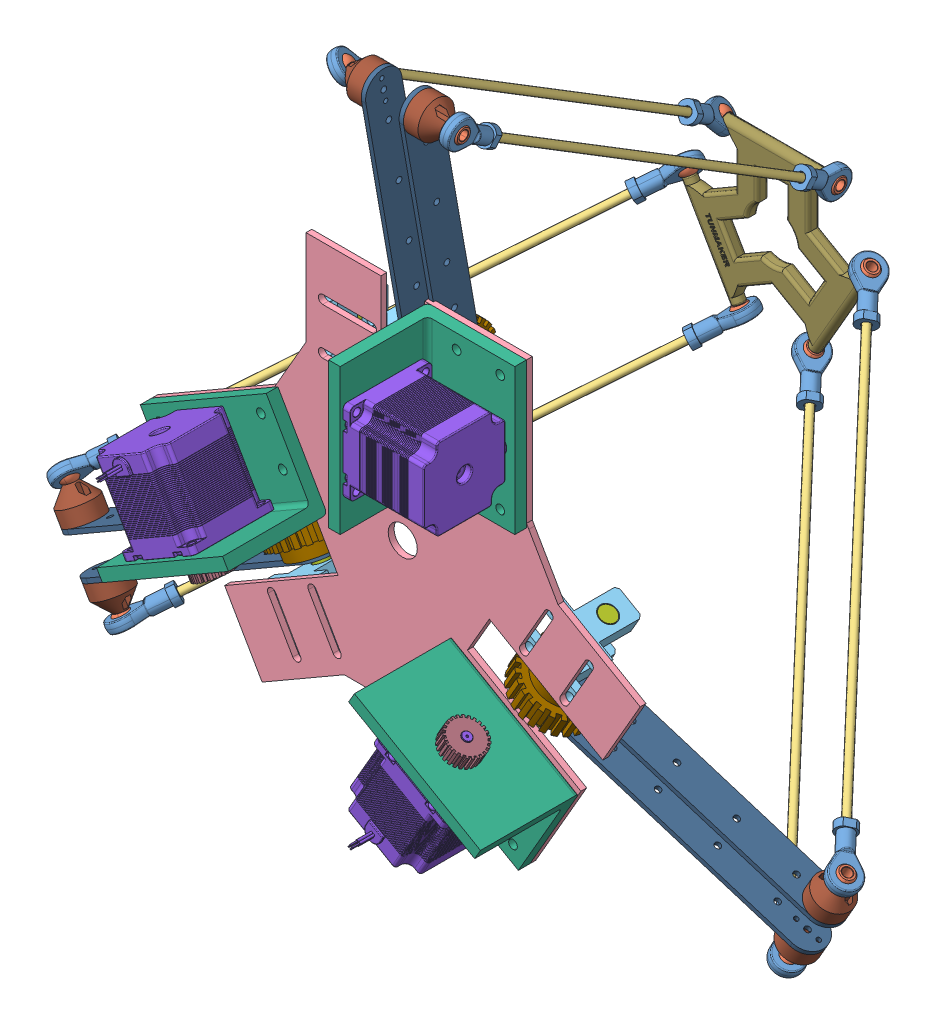
SolidWorks assembly deltabot+metal, configuration Default. Lengths in mm.
Overall size (531.43 463.37 392.64).
84 component instances, 13 part files, 0 mates.
Components (placement in the parent):
- deltabot+metal.stp-1: deltabot+metal.stp [Default] at origin size (531.43 463.37 392.64)
  - arm with joints v4.stp-1: arm with joints v4.stp [Default] at (0 -700 0) size (201.57 166.8 282.45)
    - RF_6-XE_MecMove.stp-1: RF_6-XE_MecMove.stp [Default] at (797.1961 -292.6027 -245.4013) size (39.77 32.89 44.28)
      - Component1.stp-1: Component1.stp [Default] at (-1006.4749 831.2054 216.1304) x (0.678851 0.338604 0.651543) z (0.528727 -0.841135 -0.113754) size (20 40 11)
      - Component2.stp-1: Component2.stp [Default] at (-1012.7729 825.9928 237.762) x (0.866025 0.5 0) z (-0.5 0.866025 0) size (12.7 12.7 9)
    - RF_6-XE_MecMove_1.stp-1: RF_6-XE_MecMove_1.stp [Default] at (137.5516 -501.3584 331.6266) size (39.77 32.89 44.28)
      - Component1.stp-1: Component1.stp [Default] at (-187.4437 1171.88 -595.5223) x (0.678851 0.338604 0.651543) z (-0.528727 0.841135 0.113754) size (20 40 11)
      - Component2.stp-1: Component2.stp [Default] at (-178.3751 1178.6922 -616.7328) x (0.836516 0.482963 0.258819) z (0.5 -0.866025 0) size (12.7 12.7 9)
    - connecting rod.stp-1: connecting rod.stp [Default] at (-415.8051 -153.3483 -567.1679) x (0.678851 0.338604 0.651543) z (0.509518 0.42171 -0.750034) size (5 5 300)
  - arm with joints v4_1.stp-1: arm with joints v4_1.stp [Default] at (0 -800 0) size (196.17 171.43 283.24)
    - RF_6-XE_MecMove_2.stp-1: RF_6-XE_MecMove_2.stp [Default] at (797.1961 -292.6027 -245.4013) size (34.38 37.52 45.07)
      - Component1.stp-1: Component1.stp [Default] at (-1045.4749 998.7554 216.1304) x (0.246638 0.763515 0.596837) z (0.824355 -0.489086 0.285015) size (20 40 11)
      - Component2.stp-1: Component2.stp [Default] at (-1051.7729 993.5428 237.762) x (0.866025 0.5 0) z (-0.5 0.866025 0) size (12.7 12.7 9)
    - RF_6-XE_MecMove_3.stp-1: RF_6-XE_MecMove_3.stp [Default] at (137.5516 -501.3584 331.6266) size (34.38 37.52 45.07)
      - Component1.stp-1: Component1.stp [Default] at (-226.4437 1339.43 -595.5223) x (0.246638 0.763515 0.596837) z (-0.824355 0.489086 -0.285015) size (20 40 11)
      - Component2.stp-1: Component2.stp [Default] at (-222.9163 1343.043 -592.8538) x (-0.836516 -0.482963 -0.258819) z (0.5 -0.866025 0) size (12.7 12.7 9)
    - connecting rod.stp-1: connecting rod.stp [Default] at (16.4032 -105.8427 -314.5592) x (0.246638 0.763515 0.596837) z (0.509518 0.42171 -0.750034) size (5 5 300)
  - arm with joints v4_2.stp-1: arm with joints v4_2.stp [Default] at (0 -900 0) size (236.66 169.54 252.51)
    - RF_6-XE_MecMove_4.stp-1: RF_6-XE_MecMove_4.stp [Default] at (797.1961 -292.6027 -245.4013) size (42.08 32.77 42.12)
      - Component1.stp-1: Component1.stp [Default] at (-554.93 1095.8279 187.6912) x (-0.588292 0.311209 0.746365) z (0.527669 0.847134 0.062688) size (20 40 11)
      - Component2.stp-1: Component2.stp [Default] at (-545.497 1089.4308 208.054) x (0.852869 -0.492404 -0.173648) z (0.5 0.866025 0) size (12.7 12.7 9)
    - RF_6-XE_MecMove_5.stp-1: RF_6-XE_MecMove_5.stp [Default] at (137.5516 -501.3584 331.6266) size (42.08 32.77 42.12)
      - Component1.stp-1: Component1.stp [Default] at (-86.969 1439.3187 -596.6034) x (-0.588292 0.311209 0.746365) z (-0.527669 -0.847134 -0.062688) size (20 40 11)
      - Component2.stp-1: Component2.stp [Default] at (-84.8414 1439.0413 -599.5694) x (-0.365998 0.211309 0.906308) z (-0.5 -0.866025 0) size (12.7 12.7 9)
    - connecting rod.stp-1: connecting rod.stp [Default] at (946.6115 1032.7546 -569.5657) x (-0.588292 0.311209 0.746365) z (-0.612762 0.430713 -0.662578) size (5 5 300)
  - arm with joints v4_3.stp-1: arm with joints v4_3.stp [Default] at (0 -1000 0) size (37.82 211.61 310.51)
    - RF_6-XE_MecMove_6.stp-1: RF_6-XE_MecMove_6.stp [Default] at (797.1961 -292.6027 -245.4013) size (15.43 39.54 44.57)
      - Component1.stp-1: Component1.stp [Default] at (-755.0673 1553.322 244.5695) x (0.084018 0.833371 -0.546291) z (0.993968 -0.108872 -0.013215) size (20 40 11)
      - Component2.stp-1: Component2.stp [Default] at (-754.1961 1557.8737 267.0944) x (0 -0.984808 -0.173648) z (1 0 0) size (12.7 12.7 9)
    - RF_6-XE_MecMove_7.stp-1: RF_6-XE_MecMove_7.stp [Default] at (137.5516 -501.3584 331.6266) size (15.43 39.54 44.57)
      - Component1.stp-1: Component1.stp [Default] at (-117.4731 1592.5657 -594.4413) x (0.084018 0.833371 -0.546291) z (-0.993968 0.108872 0.013215) size (20 40 11)
      - Component2.stp-1: Component2.stp [Default] at (-118.3444 1573.507 -604.7933) x (0 0 -1) z (1 0 0) size (12.7 12.7 9)
    - connecting rod.stp-1: connecting rod.stp [Default] at (511.5618 594.9454 382.7829) x (0.084018 0.833371 -0.546291) z (-0.070489 -0.541885 -0.837491) size (5 5 300)
  - arm with joints v4_4.stp-1: arm with joints v4_4.stp [Default] at (0 -1100 0) size (47.47 212.02 310.6)
    - RF_6-XE_MecMove_8.stp-1: RF_6-XE_MecMove_8.stp [Default] at (797.1961 -292.6027 -245.4013) size (25.08 39.95 44.66)
      - Component1.stp-1: Component1.stp [Default] at (-833.0673 1653.322 244.5695) x (0.753822 -0.578791 0.311051) z (-0.653287 -0.609394 0.449284) size (20 40 11)
      - Component2.stp-1: Component2.stp [Default] at (-832.1961 1662.1665 242.7486) x (0 -0.984808 -0.173648) z (-1 0 0) size (12.7 12.7 9)
    - RF_6-XE_MecMove_9.stp-1: RF_6-XE_MecMove_9.stp [Default] at (137.5516 -501.3584 331.6266) size (25.08 39.95 44.66)
      - Component1.stp-1: Component1.stp [Default] at (-195.4731 1692.5657 -594.4413) x (0.753822 -0.578791 0.311051) z (0.653287 0.609394 -0.449284) size (20 40 11)
      - Component2.stp-1: Component2.stp [Default] at (-196.3444 1673.507 -604.7933) x (0 0 -1) z (1 0 0) size (12.7 12.7 9)
    - connecting rod.stp-1: connecting rod.stp [Default] at (-931.6802 1451.4209 8.2253) x (0.753822 -0.578791 0.311051) z (-0.070489 -0.541885 -0.837491) size (5 5 300)
  - arm with joints v4_5.stp-1: arm with joints v4_5.stp [Default] at (0 -1200 0) size (236.83 168.87 252.83)
    - RF_6-XE_MecMove_10.stp-1: RF_6-XE_MecMove_10.stp [Default] at (797.1961 -292.6027 -245.4013) size (42.26 32.1 42.44)
      - Component1.stp-1: Component1.stp [Default] at (-593.93 1328.2779 187.6912) x (0.612958 -0.270161 -0.742493) z (-0.498804 -0.861103 -0.098465) size (20 40 11)
      - Component2.stp-1: Component2.stp [Default] at (-588.2147 1324.0272 183.7082) x (0.852869 -0.492404 -0.173648) z (-0.5 -0.866025 0) size (12.7 12.7 9)
    - RF_6-XE_MecMove_11.stp-1: RF_6-XE_MecMove_11.stp [Default] at (137.5516 -501.3584 331.6266) size (42.26 32.1 42.44)
      - Component1.stp-1: Component1.stp [Default] at (-125.969 1671.7687 -596.6034) x (0.612958 -0.270161 -0.742493) z (0.498804 0.861103 0.098465) size (20 40 11)
      - Component2.stp-1: Component2.stp [Default] at (-133.5432 1677.0926 -617.1539) x (-0.866025 0.5 0) z (0.5 0.866025 0) size (12.7 12.7 9)
    - connecting rod.stp-1: connecting rod.stp [Default] at (-511.4012 774.4489 423.7397) x (0.612958 -0.270161 -0.742493) z (-0.612762 0.430713 -0.662578) size (5 5 300)
  - Base.stp-1: Base.stp [Default] at origin size (335.56 298.61 4)
  - 12 mm rod alu support.stp-1: 12 mm rod alu support.stp [Default] at (98.916 13.3275 0) x (0.866025 -0.5 0) z (0 0 -1) size (42 12 35)
  - 12 mm rod alu support.stp-2: 12 mm rod alu support.stp [Default] at (-54.916 -62.8827 0) x (-0.866025 -0.5 0) z (0 0 -1) size (42 12 35)
  - 12 mm rod alu support.stp-3: 12 mm rod alu support.stp [Default] at (-80.2891 -102.9352 0) x (0.866025 0.5 0) z (0 0 -1) size (42 12 35)
  - 12 mm rod alu support.stp-4: 12 mm rod alu support.stp [Default] at (-20 121 0) x (0 -1 0) z (0 0 -1) size (42 12 35)
  - 12 mm rod alu support.stp-5: 12 mm rod alu support.stp [Default] at (-49 121 0) x (0 -1 0) z (0 0 -1) size (42 12 35)
  - 12 mm rod alu support.stp-6: 12 mm rod alu support.stp [Default] at (81.916 -16.1173 0) x (0.866025 -0.5 0) z (0 0 -1) size (42 12 35)
  - Stepper Mount.stp-1: Stepper Mount.stp [Default] at (258.4596 347.6652 0.886) x (0.866025 -0.5 0) z (0 0 1) size (100 68 68)
  - Stepper Mount.stp-2: Stepper Mount.stp [Default] at (171.8571 -397.6652 0.886) x (-0.866025 -0.5 0) z (0 0 1) size (100 68 68)
  - Stepper Mount.stp-3: Stepper Mount.stp [Default] at (-430.3167 50 0.886) x (0 1 0) z (0 0 1) size (100 68 68)
  - 12 mm axel.stp-1: 12 mm axel.stp [Default] at (-61 223.5554 -0.7002) x (0 -0.984808 -0.173648) z (0 -0.173648 0.984808) size (11 100 11)
  - 12 mm axel.stp-2: 12 mm axel.stp [Default] at (-39.8995 -21.9973 -0.7002) x (0.852869 -0.492404 -0.173648) z (0.150384 -0.086824 0.984808) size (11 100 11)
  - 12 mm axel.stp-3: 12 mm axel.stp [Default] at (-214.3814 -78.7398 -17.5515) x (0.866025 0.5 0) z (0 0 -1) size (11 100 11)
  - Stepper Motor length 56mm.stp-1: Stepper Motor length 56mm.stp [Default] at (-800.7521 882.2228 43.5) x (0.422618 0.906308 0) z (0 0 1) size (78.85 60.84 73.5)
  - Stepper Motor length 56mm.stp-2: Stepper Motor length 56mm.stp [Default] at (1164.4034 252.3603 43.5) x (0.573576 -0.819152 0) z (0 0 1) size (78.85 60.84 73.5)
  - Stepper Motor length 56mm.stp-3: Stepper Motor length 56mm.stp [Default] at (-363.6513 1334.5831 43.5) x (-0.996195 0.087156 0) z (0 0 -1) size (78.85 60.84 73.5)
  - pulley 50.stp-1: pulley 50.stp [Default] at (1 65.9551 177.8108) x (0 -0.173648 0.984808) z (-1 0 0) size (51 50.96 23)
  - pulley 50.stp-2: pulley 50.stp [Default] at (117.738 -67.3987 177.5254) x (0.150384 -0.086824 0.984808) z (0.5 0.866025 0) size (51 50.96 23)
  - pulley 50.stp-3: pulley 50.stp [Default] at (-87.0642 -50.8439 180.7174) x (0 0 1) z (0.5 -0.866025 0) size (51 50.96 23)
  - arm.stp-1: arm.stp [Default] at (242.9495 -126.4106 371.9297) x (-0.150384 0.086824 -0.984808) z (-0.5 -0.866025 0) size (25 195 3)
  - arm.stp-2: arm.stp [Default] at (103.2937 -79.2665 -447.6701) x (0.150384 -0.086824 0.984808) z (0.5 0.866025 0) size (25 195 3)
  - arm.stp-3: arm.stp [Default] at (-171.2256 -109.2494 -436.1217) x (0 0 1) z (0.5 -0.866025 0) size (25 195 3)
  - arm.stp-4: arm.stp [Default] at (18.5 273.6058 -411.9297) x (0 -0.173648 0.984808) z (-1 0 0) size (25 195 3)
  - arm.stp-5: arm.stp [Default] at (-184.2256 -86.7328 -436.1217) x (0 0 1) z (0.5 -0.866025 0) size (25 195 3)
  - arm.stp-6: arm.stp [Default] at (-7.5 273.6058 -411.9297) x (0 -0.173648 0.984808) z (-1 0 0) size (25 195 3)
  - Ball Top.stp-1: Ball Top.stp [Default] at (18.5 453.5434 278.0005) x (0 -0.984808 -0.173648) z (1 0 0) size (25 25 20)
  - Ball Top.stp-2: Ball Top.stp [Default] at (-10.5 534.1443 -179.1099) x (0 -0.984808 -0.173648) z (-1 0 0) size (25 25 20)
  - Ball Top.stp-3: Ball Top.stp [Default] at (-43.2107 -5.3178 -252.081) x (-0.866025 -0.5 0) z (-0.5 0.866025 0) size (25 25 20)
  - Ball Top.stp-4: Ball Top.stp [Default] at (-7.9022 -15.0676 -238.1503) x (0.852869 -0.492404 -0.173648) z (-0.5 -0.866025 0) size (25 25 20)
  - Ball Top.stp-5: Ball Top.stp [Default] at (-28.7107 -30.4325 212.081) x (-0.866025 -0.5 0) z (0.5 -0.866025 0) size (25 25 20)
  - Ball Top.stp-6: Ball Top.stp [Default] at (76.4003 -30.2533 218.9601) x (0.852869 -0.492404 -0.173648) z (0.5 0.866025 0) size (25 25 20)
  - End Effector.stp-1: End Effector.stp [Default] at (258.9073 -362.8437 -261.5882) x (0.5 -0.866025 0) z (0.224144 0.12941 -0.965926) size (127.66 107.11 34.84)
  - pulley 25.stp-1: pulley 25.stp [Default] at (246.644 -172.5954 56.294) x (0.866025 -0.5 0) z (-0.5 -0.866025 0) size (25 24.98 10)
  - pulley 25.stp-2: pulley 25.stp [Default] at (26.15 112.794 -156.3976) x (0 0 -1) z (1 0 0) size (25 24.98 10)
  - pulley 25.stp-3: pulley 25.stp [Default] at (73.4389 72.5954 30.706) x (0.866025 0.5 0) z (-0.5 0.866025 0) size (25 24.98 10)
